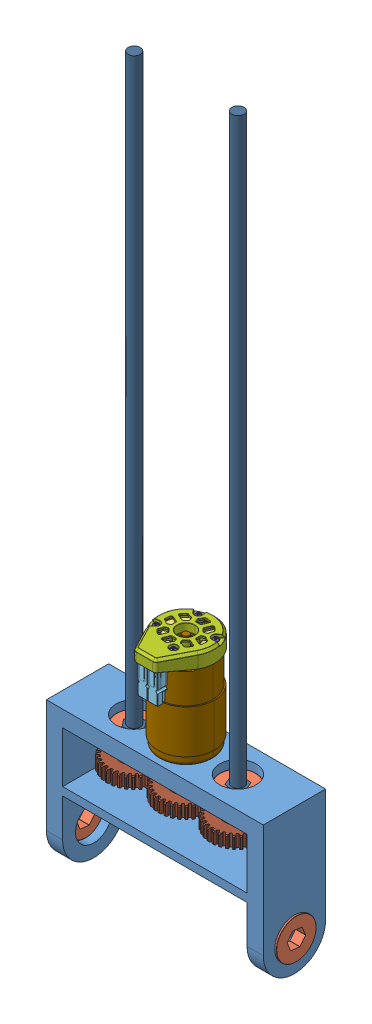
SolidWorks assembly Motor Housing Assembly, configuration Default. Lengths in mm.
Overall size (173.23 564.25 62.91).
26 component instances, 11 part files, 38 mates.
Components (placement in the parent):
- Motor housing-1: Motor housing [Default] at origin size (170.18 113.35 48.9)
- Hex Bearing-1: Hex Bearing [Default] at (-113.03 82.6033 0) x (0.99013 0 -0.140151) z (0 -1 0) size (31.12 31.12 7.93)
- Hex Bearing-2: Hex Bearing [Default] at (-72.3392 82.6033 0) x (0.454191 0 -0.890905) z (0 -1 0) size (31.12 31.12 7.93)
- 775pro.step-1: 775pro.step [Default] at (-72.39 88.9 0) x (1 0 0) z (0 -1 0) size (44.99 55.15 90.45)
  - 217-6457-000 Rev2.step-1: 217-6457-000 Rev2.step [Default] at (0 0 -66.1) x (1 0 0) z (0 1 0) size (44.99 33.26 55.15)
    - 217-6457-900 Rev1.step-1: 217-6457-900 Rev1.step [Default] at (0 5.3622 0) x (-1 0 0.000693) z (0.000693 0 1) size (41.5 28.13 51.51)
      - 217-6457-901 Rev3_Instruction Config.step-1: 217-6457-901 Rev3_Instruction Config.step [Default] at origin size (41.5 2.36 51.5)
      - 30-45BBS Rev1_SHORTENED CONTACT.step-1: 30-45BBS Rev1_SHORTENED CONTACT.step [Default] at (3.95 14.4494 26.711) x (0 1 0) z (0 0 -1) size (26 3.6 2)
      - 30-45BBS Rev1_SHORTENED CONTACT.step-2: 30-45BBS Rev1_SHORTENED CONTACT.step [Default] at (-3.9748 14.4494 26.711) x (0 1 0) z (0 0 -1) size (26 3.6 2)
      - PA45XX-X Rev1.step-1: PA45XX-X Rev1.step [Default] at (-8.4198 2.3622 73.1531) x (0 1 0) z (-1 0 0) size (24.71 8.41 8.41)
      - PA45XX-X Rev1.step-2: PA45XX-X Rev1.step [Default] at (-0.495 2.3622 73.1531) x (0 1 0) z (-1 0 0) size (24.71 8.41 8.41)
    - 217-6457-001 Rev4.step-1: 217-6457-001 Rev4.step [Default] at origin size (41.49 7.8 41.49)
    - 217-6457-002 Rev7.step-1: 217-6457-002 Rev7.step [Default] at (0 0.05 0) size (44.99 11.5 55.15)
    - 217-9191-008 Rev1.step-1: 217-9191-008 Rev1.step [Default] at (81.4247 7.8 32.3804) x (-0.560945 0 -0.827853) z (0 1 0) size (4.2 4.2 11.81)
    - 217-9191-008 Rev1.step-2: 217-9191-008 Rev1.step [Default] at (32.3804 7.8 -81.4247) x (-0.827853 0 0.560945) z (0 1 0) size (4.2 4.2 11.81)
    - 217-9191-008 Rev1.step-3: 217-9191-008 Rev1.step [Default] at (-81.4247 7.8 -32.3804) x (0.560945 0 0.827853) z (0 1 0) size (4.2 4.2 11.81)
    - 217-9191-008 Rev1.step-4: 217-9191-008 Rev1.step [Default] at (-32.3804 7.8 81.4247) x (0.827853 0 -0.560945) z (0 1 0) size (4.2 4.2 11.81)
  - 217-4347-000 Rev2.step-1: 217-4347-000 Rev2.step [Default] x (0 0 -1) z (-1 0 0) size (88 44.3 44.3)
- Hex Bearing-3: Hex Bearing [Default] at (6.2967 0 0) x (0 -0.924225 -0.381849) z (1 0 0) size (31.12 31.12 7.93)
- Hex Bearing-4: Hex Bearing [Default] at (-151.0767 0 0) x (0 0.924225 0.381849) z (-1 0 0) size (31.12 31.12 7.93)
- Hex Bearing-5: Hex Bearing [Default] at (-31.6484 82.6033 0) x (-0.99013 0 -0.140151) z (0 -1 0) size (31.12 31.12 7.93)
- Lead Screw to Hex Axle-2: Lead Screw to Hex Axle [Default] at (-31.6829 50.8533 -0.0857) x (-0.373691 0 -0.927553) z (0 1 0) size (14.66 12.7 488.95)
- REV-21-1927.step-1: REV-21-1927.step [Default] at (-113.03 57.2033 0) x (0.787403 0 -0.616439) z (0 1 0) size (43.11 43.11 12.7)
- REV-21-1927.step-2: REV-21-1927.step [Default] at (-72.3392 57.2033 0) x (0.086983 0 -0.99621) z (0 1 0) size (43.11 43.11 12.7)
- REV-21-1927.step-3: REV-21-1927.step [Default] at (-31.6484 57.2033 0) x (0.927553 0 -0.373691) z (0 1 0) size (43.11 43.11 12.7)
- Lead Screw to Hex Axle-4: Lead Screw to Hex Axle [Default] at (-113.03 50.8533 0) x (0.616439 0 0.787403) z (0 1 0) size (14.66 12.7 488.95)
Mates (geometry in assembly coordinates):
- Concentric1: concentric anti-aligned: circle of Motor housing-1; circle of REV-21-1928.step-1
- Distance1: distance = 11.43 mm anti-aligned: plane of REV-21-1928.step-1 through (-115.57 64.77 0) normal (0 1 0); plane of Motor housing-1 through (-144.78 76.2 -24.4475) normal (0 -1 0)
- Concentric2: concentric anti-aligned: circle of Motor housing-1; circle of REV-21-1928.step-2
- Distance2: distance = 11.43 mm anti-aligned: plane of REV-21-1928.step-2 through (-72.3392 64.77 0) normal (0 1 0); plane of Motor housing-1 through (-144.78 76.2 -24.4475) normal (0 -1 0)
- Coincident3: coincident anti-aligned: plane of Motor housing-1 through (-144.78 76.2 -24.4475) normal (0 -1 0); plane of Hex Bearing-1 through (-99.1979 76.2 -1.9579) normal (0 1 0)
- Concentric3: concentric aligned: cylinder of Motor housing-1 through (-113.03 63.246 0) axis (0 1 0) radius 14.2875; cylinder of Hex Bearing-1 through (-113.03 74.676 0) axis (0 1 0) radius 14.2875
- Coincident4: coincident anti-aligned: plane of Motor housing-1 through (-144.78 76.2 -24.4475) normal (0 -1 0); plane of Hex Bearing-2 through (-65.9942 76.2 -12.4459) normal (0 1 0)
- Concentric4: concentric aligned: cylinder of Motor housing-1 through (-72.3392 63.246 0) axis (0 1 0) radius 14.2875; cylinder of Hex Bearing-2 through (-72.3392 74.676 0) axis (0 1 0) radius 14.2875
- Coincident6: coincident anti-aligned: plane of Motor housing-1 through (12.7 88.9 -24.4475) normal (0 1 0); plane of 775pro.step-1/217-4347-000 Rev2.step-1 through (-72.39 88.9 -8.75) normal (0 -1 0)
- Coincident7: coincident anti-aligned: plane of REV-21-1928.step-2 through (-67.894 64.7815 -5.8313) normal (-0.922661 0 0.385613); plane of Lead Screw to Hex Axle-1 through (-75.6695 83.82 6.5324) normal (0.052112 0 0.998641)
- Coincident8: coincident anti-aligned: plane of REV-21-1928.step-2 through (-65.0666 64.7815 0.934) normal (-0.795281 0 -0.606241); plane of Lead Screw to Hex Axle-1 through (-79.6616 83.82 0.3821) normal (-0.838793 0 0.544451)
- Coincident9: coincident aligned: plane of REV-21-1928.step-2 through (-72.3392 52.07 0) normal (0 -1 0); plane of Lead Screw to Hex Axle-1 through (-72.3392 52.07 0) normal (0 -1 0)
- Coincident10: coincident anti-aligned: plane of Hex Bearing-2 through (-68.3471 74.676 6.1503) normal (-0.890905 0 -0.454191); plane of Lead Screw to Hex Axle-1 through (-68.3471 83.82 6.1503) normal (0.890905 0 0.454191)
- Concentric6: concentric aligned: cylinder of Motor housing-1 through (12.7 0 0) axis (-1 0 0) radius 14.2875; cylinder of Hex Bearing-3 through (14.224 0 0) axis (-1 0 0) radius 14.2875
- Coincident11: coincident anti-aligned: plane of Motor housing-1 through (12.7 0 0) normal (1 0 0); plane of Hex Bearing-3 through (12.7 -12.9114 -5.3344) normal (-1 0 0)
- Concentric7: concentric aligned: cylinder of Motor housing-1 through (-157.48 0 0) axis (1 0 0) radius 14.2875; cylinder of Hex Bearing-4 through (-159.004 0 0) axis (1 0 0) radius 14.2875
- Coincident12: coincident anti-aligned: plane of Motor housing-1 through (-157.48 0 0) normal (-1 0 0); plane of Hex Bearing-4 through (-157.48 12.9114 5.3344) normal (1 0 0)
- GearMate1: gear = 25.4 : 25.4 mm: circle of REV-21-1928.step-1; circle of REV-21-1928.step-2
- Concentric8: concentric anti-aligned: circle of Motor housing-1; circle of REV-21-1928.step-3
- Coincident14: coincident aligned: plane of REV-21-1928.step-2 through (-72.3392 64.77 0) normal (0 1 0); plane of REV-21-1928.step-3 through (-29.1084 64.77 0) normal (0 1 0)
- GearMate2: gear = 25.4 : 25.4 mm: circle of REV-21-1928.step-2; circle of REV-21-1928.step-3
- Concentric9: concentric aligned: cylinder of Motor housing-1 through (-31.6484 63.246 0) axis (0 1 0) radius 14.2875; cylinder of Hex Bearing-5 through (-31.6484 74.676 0) axis (0 1 0) radius 14.2875
- Coincident15: coincident anti-aligned: plane of Motor housing-1 through (-144.78 76.2 -24.4475) normal (0 -1 0); plane of Hex Bearing-5 through (-45.4805 76.2 -1.9579) normal (0 1 0)
- Coincident16: coincident anti-aligned: plane of REV-21-1928.step-3 through (-34.9129 64.7815 4.48) normal (0.991073 0 -0.133321); plane of Lead Screw to Hex Axle-2 through (-38.9429 82.6033 -1.1133) normal (-0.927553 0 0.373691)
- Coincident17: coincident anti-aligned: plane of REV-21-1928.step-3 through (-28.1308 64.7815 7.2669) normal (0.380077 0 -0.924955); plane of Lead Screw to Hex Axle-2 through (-36.2029 82.6033 5.6878) normal (-0.140151 0 0.99013)
- Coincident18: coincident aligned: plane of REV-21-1928.step-3 through (-29.1084 52.07 0) normal (0 -1 0); plane of Lead Screw to Hex Axle-2 through (-31.6829 50.8533 -0.0857) normal (0 -1 0)
- Coincident23: coincident anti-aligned: plane of Hex Bearing-5 through (-38.9084 74.676 -1.0276) normal (0.927553 0 -0.373691); plane of Lead Screw to Hex Axle-2 through (-38.9429 82.6033 -1.1133) normal (-0.927553 0 0.373691)
- Concentric10: concentric anti-aligned: circle of Motor housing-1; circle of REV-21-1927.step-1
- Concentric11: concentric anti-aligned: circle of Motor housing-1; circle of REV-21-1927.step-3
- Coincident28: coincident anti-aligned: plane of Lead Screw to Hex Axle-2 through (-38.9429 82.6033 -1.1133) normal (-0.927553 0 0.373691); plane of REV-21-1927.step-3 through (-36.1683 63.5649 5.7735) normal (0.927553 0 -0.373691)
- Coincident29: coincident aligned: plane of Lead Screw to Hex Axle-2 through (-31.6829 50.8533 -0.0857) normal (0 -1 0); plane of REV-21-1927.step-3 through (-31.6484 50.8533 0) normal (0 -1 0)
- Concentric12: concentric anti-aligned: circle of Motor housing-1; circle of REV-21-1927.step-2
- Coincident30: coincident aligned: plane of REV-21-1927.step-2 through (-72.3392 50.8533 0) normal (0 -1 0); plane of REV-21-1927.step-3 through (-31.6484 50.8533 0) normal (0 -1 0)
- GearMate3: gear = 25.4 : 25.4 mm: circle of REV-21-1927.step-2; circle of REV-21-1927.step-3
- GearMate4: gear = 25.4 : 25.4 mm: circle of REV-21-1927.step-2; circle of REV-21-1927.step-1
- Coincident31: coincident anti-aligned: plane of Hex Bearing-1 through (-105.77 74.676 -1.0276) normal (-0.787403 0 0.616439); plane of Lead Screw to Hex Axle-4 through (-105.77 82.6033 -1.0276) normal (0.787403 0 -0.616439)
- Coincident32: coincident anti-aligned: plane of Hex Bearing-1 through (-110.29 74.676 -6.8011) normal (0.140151 0 0.99013); plane of Lead Screw to Hex Axle-4 through (-110.29 82.6033 -6.8011) normal (-0.140151 0 -0.99013)
- Coincident33: coincident aligned: plane of Hex Bearing-1 through (-113.03 82.6033 0) normal (0 1 0); plane of Lead Screw to Hex Axle-4 through (-113.03 82.6033 0) normal (0 1 0)
